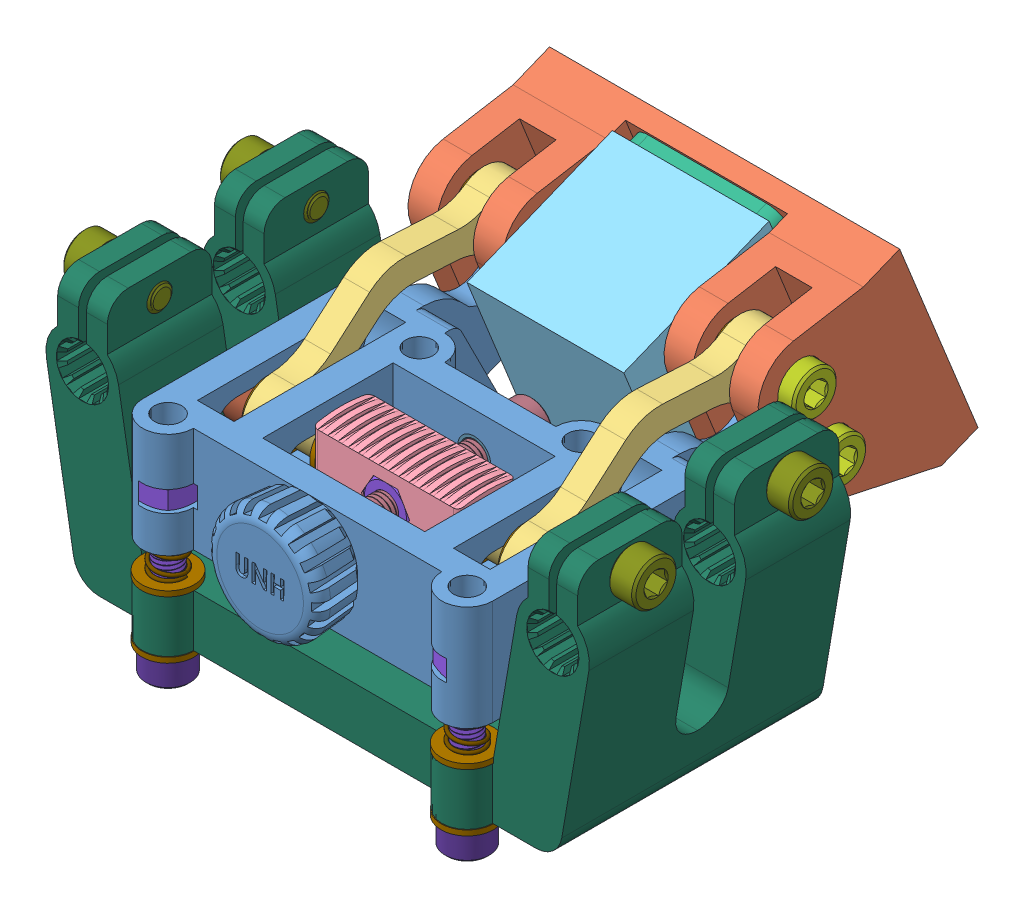
SolidWorks assembly Camera_Angle_Assembly_M5, configuration Default. Lengths in mm.
Overall size (109.96 65.35 103.86).
86 component instances, 19 part files, 86 mates.
Components (placement in the parent):
- Body_Bracket_M5-1: Body_Bracket_M5 [Default] at (-16.3834 -2.0346 -10.9973) size (67 20.14 76.95)
- Camera_Swing_Bracket_M5-1: Camera_Swing_Bracket_M5 [Default] at (-16.3834 -14.0182 -34.7174) x (1 0 0) z (0 -0.374784 0.927112) size (67 43.1 30.6)
- 42-72mm_Linkage_bent_angle_M5-1: 42-72mm_Linkage_bent_angle_M5 [Default] at (-9.8834 11.872 -5.3755) x (1 0 0) z (0 -0.325531 0.945531) size (5 16.61 54.86)
- 42-72mm_Linkage_bent_angle_M5-2: 42-72mm_Linkage_bent_angle_M5 [Default] at (-58.8834 11.872 -5.3755) x (1 0 0) z (0 -0.325531 0.945531) size (5 16.61 54.86)
- Sled_Block_M5-1: Sled_Block_M5 [Default] at (-31.8834 -2.0346 29.5176) size (28 13.83 11)
- Camera_Appr-1: Camera_Appr [Default] at (-17.3834 11.8179 9.4336) x (-1 0 0) z (0 -0.374784 0.927112) size (30 50 30)
- Adapter_Appr-1: Adapter_Appr [Default] at (-46.3834 -14.0231 -33.3711) x (0 0.927112 0.374784) z (-1 0 0) size (39 2.5 29)
- Pivot_Joints-1: Pivot_Joints [Default] at (-19.4217 -14.2043 8.9956) x (0 0.138984 0.990295) z (-1 0 0) size (10 10 21.93)
  - 16mm_M5x0-8-1: 16mm_M5x0-8 [91292A126] at (-10.6074 27.8206 -3.0383) size (8.5 8.5 21.93)
  - 8mm_M5x0-8_Nut-1: 8mm_M5x0-8_Nut [91828A241] at (-10.6074 27.8206 -5.0383) size (8 9.24 4.46)
  - 5-3_IDx10mm_OD_Washer-1: 5-3_IDx10mm_OD_Washer [93475A240] at (-10.6074 27.8206 -9.5383) size (10 10 1)
  - 5-3_IDx10mm_OD_Washer-2: 5-3_IDx10mm_OD_Washer [93475A240] at (-10.6074 27.8206 -15.5383) size (10 10 1)
  - 5mm_Bushing-1: 5mm_Bushing [Default] at (-10.6074 27.8206 -14.5383) size (6.35 6.35 5)
- Pivot_Joints-2: Pivot_Joints [Default] at (-19.4217 -28.111 3.3738) x (0 0.138984 0.990295) z (-1 0 0) size (10 10 21.93)
  - 16mm_M5x0-8-1: 16mm_M5x0-8 [91292A126] at (-10.6074 27.8206 -3.0383) size (8.5 8.5 21.93)
  - 8mm_M5x0-8_Nut-1: 8mm_M5x0-8_Nut [91828A241] at (-10.6074 27.8206 -5.0383) size (8 9.24 4.46)
  - 5-3_IDx10mm_OD_Washer-1: 5-3_IDx10mm_OD_Washer [93475A240] at (-10.6074 27.8206 -9.5383) size (10 10 1)
  - 5-3_IDx10mm_OD_Washer-2: 5-3_IDx10mm_OD_Washer [93475A240] at (-10.6074 27.8206 -15.5383) size (10 10 1)
  - 5mm_Bushing-1: 5mm_Bushing [Default] at (-10.6074 27.8206 -14.5383) size (6.35 6.35 5)
- Pivot_Joints-3: Pivot_Joints [Default] at (-44.3451 -17.1529 -12.0134) x (0 -0.138984 -0.990295) z (1 0 0) size (10 10 21.93)
  - 16mm_M5x0-8-1: 16mm_M5x0-8 [91292A126] at (-10.6074 27.8206 -3.0383) size (8.5 8.5 21.93)
  - 8mm_M5x0-8_Nut-1: 8mm_M5x0-8_Nut [91828A241] at (-10.6074 27.8206 -5.0383) size (8 9.24 4.46)
  - 5-3_IDx10mm_OD_Washer-1: 5-3_IDx10mm_OD_Washer [93475A240] at (-10.6074 27.8206 -9.5383) size (10 10 1)
  - 5-3_IDx10mm_OD_Washer-2: 5-3_IDx10mm_OD_Washer [93475A240] at (-10.6074 27.8206 -15.5383) size (10 10 1)
  - 5mm_Bushing-1: 5mm_Bushing [Default] at (-10.6074 27.8206 -14.5383) size (6.35 6.35 5)
- Pivot_Joints-4: Pivot_Joints [Default] at (-44.3451 -22.2956 10.8201) x (0 -0.927112 -0.374784) z (1 0 0) size (10 10 21.93)
  - 16mm_M5x0-8-1: 16mm_M5x0-8 [91292A126] at (-10.6074 27.8206 -3.0383) size (8.5 8.5 21.93)
  - 8mm_M5x0-8_Nut-1: 8mm_M5x0-8_Nut [91828A241] at (-10.6074 27.8206 -5.0383) size (8 9.24 4.46)
  - 5-3_IDx10mm_OD_Washer-1: 5-3_IDx10mm_OD_Washer [93475A240] at (-10.6074 27.8206 -9.5383) size (10 10 1)
  - 5-3_IDx10mm_OD_Washer-2: 5-3_IDx10mm_OD_Washer [93475A240] at (-10.6074 27.8206 -15.5383) size (10 10 1)
  - 5mm_Bushing-1: 5mm_Bushing [Default] at (-10.6074 27.8206 -14.5383) size (6.35 6.35 5)
- 8mm_M5x0-8_Nut-1: 8mm_M5x0-8_Nut [91828A241] at (-31.8834 -2.0346 38.5176) x (0.866025 -0.5 0) z (0 0 1) size (8 9.24 4.46)
- 8mm_M5x0-8_Nut-2: 8mm_M5x0-8_Nut [91828A241] at (-31.8834 -2.0346 31.5176) x (0.866025 0.5 0) z (0 0 1) size (8 9.24 4.46)
- 8mm_M5x0-8_Nut-3: 8mm_M5x0-8_Nut [91828A241] at (-43.8834 -2.0346 35.0176) x (0 -0.866025 -0.5) z (1 0 0) size (8 9.24 4.46)
- 8mm_M5x0-8_Nut-4: 8mm_M5x0-8_Nut [91828A241] at (-19.8834 -2.0346 35.0176) x (0 -0.866025 0.5) z (-1 0 0) size (8 9.24 4.46)
- 5-3_IDx10mm_OD_Washer-1: 5-3_IDx10mm_OD_Washer [93475A240] at (-31.8834 -2.0346 52.5027) x (-0.658072 -0.752955 0) z (0 0 1) size (10 10 1)
- 5-3_IDx10mm_OD_Washer-2: 5-3_IDx10mm_OD_Washer [93475A240] at (-31.8834 -2.0346 18.5527) size (10 10 1)
- Slider_Bolt_Assembly_M5-1: Slider_Bolt_Assembly_M5 [Default] at (-13.1473 -15.2033 38.4623) x (0 -0.5 0.866025) z (-1 0 0) size (13.73 13.73 25.93)
  - 20mm_M5x0-8-1: 20mm_M5x0-8 [91292A128] at (-9.5676 9.6821 10.7361) size (8.5 8.5 25.93)
  - 5-3_IDx10mm_OD_Washer-1: 5-3_IDx10mm_OD_Washer [93475A240] at (-9.5676 9.6821 -9.2639) size (10 10 1)
  - 5mm_Bushing-3: 5mm_Bushing [Default] at (-9.5676 9.6821 -8.2639) size (6.35 6.35 5)
  - 5-3_IDx10mm_OD_Washer-2: 5-3_IDx10mm_OD_Washer [93475A240] at (-9.5676 9.6821 -3.2639) x (0.855536 0.517743 0) z (0 0 1) size (10 10 1)
  - 6mm_Bushing-2: 6mm_Bushing [Default] at (-9.5676 9.6821 -2.2639) x (-0.990313 -0.138856 0) z (0 0 1) size (6.35 6.35 6)
  - 5-3_IDx10mm_OD_Washer-3: 5-3_IDx10mm_OD_Washer [93475A240] at (-9.5676 9.6821 3.7361) x (0.855536 0.517743 0) z (0 0 1) size (10 10 1)
- Slider_Bolt_Assembly_M5-2: Slider_Bolt_Assembly_M5 [Default] at (-50.6195 -11.6022 44.6996) x (0 -1 0) z (1 0 0) size (13.73 13.73 25.93)
  - 20mm_M5x0-8-1: 20mm_M5x0-8 [91292A128] at (-9.5676 9.6821 10.7361) size (8.5 8.5 25.93)
  - 5-3_IDx10mm_OD_Washer-1: 5-3_IDx10mm_OD_Washer [93475A240] at (-9.5676 9.6821 -9.2639) size (10 10 1)
  - 5mm_Bushing-3: 5mm_Bushing [Default] at (-9.5676 9.6821 -8.2639) size (6.35 6.35 5)
  - 5-3_IDx10mm_OD_Washer-2: 5-3_IDx10mm_OD_Washer [93475A240] at (-9.5676 9.6821 -3.2639) x (0.855536 0.517743 0) z (0 0 1) size (10 10 1)
  - 6mm_Bushing-2: 6mm_Bushing [Default] at (-9.5676 9.6821 -2.2639) x (-0.990313 -0.138856 0) z (0 0 1) size (6.35 6.35 6)
  - 5-3_IDx10mm_OD_Washer-3: 5-3_IDx10mm_OD_Washer [93475A240] at (-9.5676 9.6821 3.7361) x (0.855536 0.517743 0) z (0 0 1) size (10 10 1)
- 45mm_M5x0-8_Bolt-1: 45mm_M5x0-8_Bolt [91290A197] at (-31.8834 -2.0346 62.5527) x (-0.070148 -0.997537 0) z (0 0 1) size (8.5 8.5 50.62)
- 4mm_Bushing-1: 4mm_Bushing [Default] at (-31.8834 -2.0346 19.5527) x (0.999697 0.024604 0) z (0 0 1) size (6.35 6.35 4)
- 4mm_Bushing-2: 4mm_Bushing [Default] at (-31.8834 -2.0346 48.5027) x (0.999452 0.033088 0) z (0 0 1) size (6.35 6.35 4)
- 5-3_IDx10mm_OD_Washer-3: 5-3_IDx10mm_OD_Washer [93475A240] at (-31.8834 -2.0346 53.5027) x (-0.658072 -0.752955 0) z (0 0 1) size (10 10 1)
- 5-3_IDx10mm_OD_Washer-4: 5-3_IDx10mm_OD_Washer [93475A240] at (-31.8834 -2.0346 17.5527) x (-0.656863 -0.75401 0) z (0 0 1) size (10 10 1)
- Mounting_Plate_M5-1: Mounting_Plate_M5 [Default] at (-31.8834 -31.3046 30.9402) x (-1 0 0) z (0 0 -1) size (104 49.82 55.08)
- 10mm_M5x0-8_Bolt-1: 10mm_M5x0-8_Bolt [91292A124] at (7.8666 14.0165 43.5027) x (0 -0.230781 0.973006) z (-1 0 0) size (8.5 8.5 15.93)
- 10mm_M5x0-8_Bolt-2: 10mm_M5x0-8_Bolt [91292A124] at (7.8666 14.0165 13.5027) x (0 -0.230781 0.973006) z (-1 0 0) size (8.5 8.5 15.93)
- 10mm_M5x0-8_Bolt-3: 10mm_M5x0-8_Bolt [91292A124] at (-71.6334 14.0165 13.5027) x (0 -0.230781 -0.973006) z (1 0 0) size (8.5 8.5 15.93)
- 10mm_M5x0-8_Bolt-4: 10mm_M5x0-8_Bolt [91292A124] at (-71.6334 14.0165 43.5027) x (0 -0.230781 -0.973006) z (1 0 0) size (8.5 8.5 15.93)
- Spring_Tilt_Bolt-1: Spring_Tilt_Bolt [Default] at (-40.1833 -35.3156 43.4609) x (0.983923 0 -0.178593) z (0 1 0) size (11.84 12.15 35.93)
  - 30mm_M5x0-8_Bolt-1: 30mm_M5x0-8_Bolt [91292A192] at (-21.7917 -6.2505 33.0109) size (8.5 8.5 35.93)
  - 5-3_IDx10mm_OD_Washer-1: 5-3_IDx10mm_OD_Washer [93475A240] at (-21.7917 -6.2505 3.0109) size (10 10 1)
  - Spring-1: Spring [9657K272] at (-21.7731 -6.2413 27.7109) size (6.54 6.63 13.03)
  - 5-3_IDx10mm_OD_Washer-2: 5-3_IDx10mm_OD_Washer [93475A240] at (-21.7917 -6.2505 14.0109) x (0.999587 -0.028726 0) z (0 0 1) size (10 10 1)
  - 8mm_M5x0-8_Nut-1: 8mm_M5x0-8_Nut [91828A241] at (-21.7917 -6.2505 29.7109) x (0.822023 0.569454 0) z (0 0 1) size (8 9.24 4.46)
- Spring_Tilt_Bolt-2: Spring_Tilt_Bolt [Default] at (-13.3002 -35.3156 33.1776) x (-0.178593 0 -0.983923) z (0 1 0) size (11.84 12.15 35.93)
  - 30mm_M5x0-8_Bolt-1: 30mm_M5x0-8_Bolt [91292A192] at (-21.7917 -6.2505 33.0109) size (8.5 8.5 35.93)
  - 5-3_IDx10mm_OD_Washer-1: 5-3_IDx10mm_OD_Washer [93475A240] at (-21.7917 -6.2505 3.0109) size (10 10 1)
  - Spring-1: Spring [9657K272] at (-21.7731 -6.2413 27.7109) size (6.54 6.63 13.03)
  - 5-3_IDx10mm_OD_Washer-2: 5-3_IDx10mm_OD_Washer [93475A240] at (-21.7917 -6.2505 14.0109) x (0.999587 -0.028726 0) z (0 0 1) size (10 10 1)
  - 8mm_M5x0-8_Nut-1: 8mm_M5x0-8_Nut [91828A241] at (-21.7917 -6.2505 29.7109) x (0.822023 0.569454 0) z (0 0 1) size (8 9.24 4.46)
- Spring_Tilt_Bolt-3: Spring_Tilt_Bolt [Default] at (-25.9107 -35.3156 25.8241) x (0.822023 0 0.569454) z (0 1 0) size (11.84 12.15 35.93)
  - 30mm_M5x0-8_Bolt-1: 30mm_M5x0-8_Bolt [91292A192] at (-21.7917 -6.2505 33.0109) size (8.5 8.5 35.93)
  - 5-3_IDx10mm_OD_Washer-1: 5-3_IDx10mm_OD_Washer [93475A240] at (-21.7917 -6.2505 3.0109) size (10 10 1)
  - Spring-1: Spring [9657K272] at (-21.7731 -6.2413 27.7109) size (6.54 6.63 13.03)
  - 5-3_IDx10mm_OD_Washer-2: 5-3_IDx10mm_OD_Washer [93475A240] at (-21.7917 -6.2505 14.0109) x (0.999587 -0.028726 0) z (0 0 1) size (10 10 1)
  - 8mm_M5x0-8_Nut-1: 8mm_M5x0-8_Nut [91828A241] at (-21.7917 -6.2505 29.7109) x (0.822023 0.569454 0) z (0 0 1) size (8 9.24 4.46)
- Spring_Tilt_Bolt-4: Spring_Tilt_Bolt [Default] at (-20.8225 -35.3156 -3.6789) x (0.082151 0 -0.99662) z (0 1 0) size (11.84 12.15 35.93)
  - 30mm_M5x0-8_Bolt-1: 30mm_M5x0-8_Bolt [91292A192] at (-21.7917 -6.2505 33.0109) size (8.5 8.5 35.93)
  - 5-3_IDx10mm_OD_Washer-1: 5-3_IDx10mm_OD_Washer [93475A240] at (-21.7917 -6.2505 3.0109) size (10 10 1)
  - Spring-1: Spring [9657K272] at (-21.7731 -6.2413 27.7109) size (6.54 6.63 13.03)
  - 5-3_IDx10mm_OD_Washer-2: 5-3_IDx10mm_OD_Washer [93475A240] at (-21.7917 -6.2505 14.0109) x (0.999587 -0.028726 0) z (0 0 1) size (10 10 1)
  - 8mm_M5x0-8_Nut-1: 8mm_M5x0-8_Nut [91828A241] at (-21.7917 -6.2505 29.7109) x (0.822023 0.569454 0) z (0 0 1) size (8 9.24 4.46)
- Knob-1: Knob [Default] at (-31.8834 -2.0346 54.5027) x (0.999929 -0.011934 0) z (0 0 1) size (21.77 21.77 10)
Mates (geometry in assembly coordinates):
- Distance2: distance = 1 mm anti-aligned: plane of Camera_Swing_Bracket_M5-1 through (-10.8834 -14.0182 -34.7174) normal (1 0 0); plane of Body_Bracket_M5-1 through (-9.8834 -2.0346 -10.9973) normal (-1 0 0)
- Distance3: distance = 1 mm anti-aligned: plane of 42-72mm_Linkage_bent_angle_M5-1 through (-4.8834 14.025 35.5957) normal (1 0 0); plane of Camera_Swing_Bracket_M5-1 through (-3.8834 -14.0182 -34.7174) normal (-1 0 0)
- Slot1: slot aligned: cylinder of 42-72mm_Linkage_bent_angle_M5-1 through (-4.8834 -2.0346 35.0176) axis (-1 0 0) radius 3.175; plane of Body_Bracket_M5-1 through (1.6166 -5.2096 41.0027) normal (0 1 0); cylinder of Body_Bracket_M5-1 through (1.6166 -2.0346 29.0027) axis (-1 0 0) radius 3.175
- Concentric3: concentric anti-aligned: circle of Camera_Swing_Bracket_M5-1; circle of 42-72mm_Linkage_bent_angle_M5-2
- Concentric4: concentric aligned: circle of 42-72mm_Linkage_bent_angle_M5-1; circle of 42-72mm_Linkage_bent_angle_M5-2
- Distance4: distance = 1 mm anti-aligned: plane of 42-72mm_Linkage_bent_angle_M5-2 through (-58.8834 14.025 35.5957) normal (-1 0 0); plane of Camera_Swing_Bracket_M5-1 through (-59.8834 -14.0182 -34.7174) normal (1 0 0)
- Concentric6: concentric anti-aligned: circle of Body_Bracket_M5-1; circle of Sled_Block_M5-1
- Concentric7: concentric anti-aligned: circle of Camera_Swing_Bracket_M5-1; circle of Adapter_Appr-1
- Parallel1: parallel anti-aligned: plane of Camera_Swing_Bracket_M5-1 through (1.6166 -2.0346 -10.9973) normal (1 0 0); plane of Adapter_Appr-1 through (-46.3834 -10.1194 -34.4896) normal (-1 0 0)
- Coincident1: coincident anti-aligned: plane of Camera_Swing_Bracket_M5-1 through (-31.8834 -13.5497 -35.8763) normal (0 -0.374784 0.927112); plane of Adapter_Appr-1 through (-43.1834 -10.1194 -34.4896) normal (0 0.374784 -0.927112)
- Coincident2: coincident anti-aligned: plane of Camera_Appr-1 through (-17.3834 -14.0231 -33.3711) normal (0 0.374784 -0.927112); plane of Adapter_Appr-1 through (-43.1834 -11.0563 -32.1718) normal (0 -0.374784 0.927112)
- Coincident3: coincident aligned: plane of Camera_Appr-1 through (-17.3834 -25.2666 -5.5578) normal (1 0 0); plane of Adapter_Appr-1 through (-17.3834 -10.1194 -34.4896) normal (1 0 0)
- Coincident4: coincident aligned: plane of Camera_Appr-1 through (-17.3834 -25.2666 -5.5578) normal (0 -0.927112 -0.374784); plane of Adapter_Appr-1 through (-43.1834 -13.0861 -35.6889) normal (0 -0.927112 -0.374784)
- LimitAngle3: limit planar angle = 1.95496 rad anti-aligned: plane of Camera_Swing_Bracket_M5-1 through (1.6166 -12.1443 -39.353) normal (0 0.374784 -0.927112); plane of Body_Bracket_M5-1 through (1.6166 5.5354 13.4839) normal (0 1 0)
- Concentric8: concentric aligned: circle of Camera_Swing_Bracket_M5-1; circle of 42-72mm_Linkage_bent_angle_M5-1
- Concentric9: concentric aligned: circle of Body_Bracket_M5-1; circle of Camera_Swing_Bracket_M5-1
- Concentric10: concentric anti-aligned: circle of Camera_Swing_Bracket_M5-1; circle of Pivot_Joints-1/5-3_IDx10mm_OD_Washer-2
- Coincident5: coincident anti-aligned: plane of Camera_Swing_Bracket_M5-1 through (-0.3834 11.872 -5.3755) normal (1 0 0); plane of Pivot_Joints-1/16mm_M5x0-8-1 through (-0.3834 11.872 -5.3755) normal (-1 0 0)
- Coincident6: coincident anti-aligned: plane of Camera_Swing_Bracket_M5-1 through (-12.3834 13.6031 -9.6577) normal (0 -0.788128 0.615511); plane of Pivot_Joints-1/8mm_M5x0-8_Nut-1 through (-16.3834 16.446 -6.0175) normal (0 0.788128 -0.615511)
- Concentric11: concentric aligned: circle of Camera_Swing_Bracket_M5-1; circle of Pivot_Joints-2/16mm_M5x0-8-1
- Coincident7: coincident anti-aligned: circle of Camera_Swing_Bracket_M5-1; plane of Pivot_Joints-2/16mm_M5x0-8-1 through (-0.3834 -2.0346 -10.9973) normal (-1 0 0)
- Parallel2: parallel anti-aligned: plane of Camera_Swing_Bracket_M5-1 through (-12.3834 -4.8776 -14.6375) normal (0 0.138984 0.990295); plane of Pivot_Joints-2/8mm_M5x0-8_Nut-1 through (-16.3834 -0.3036 -15.2794) normal (0 -0.138984 -0.990295)
- Concentric12: concentric aligned: circle of Camera_Swing_Bracket_M5-1; circle of Pivot_Joints-3/5-3_IDx10mm_OD_Washer-2
- Coincident8: coincident anti-aligned: plane of Camera_Swing_Bracket_M5-1 through (-63.3834 11.872 -5.3755) normal (-1 0 0); plane of Pivot_Joints-3/16mm_M5x0-8-1 through (-63.3834 11.872 -5.3755) normal (1 0 0)
- Parallel3: parallel anti-aligned: plane of Camera_Swing_Bracket_M5-1 through (-51.3834 13.6031 -9.6577) normal (0 -0.788128 0.615511); plane of Pivot_Joints-3/8mm_M5x0-8_Nut-1 through (-47.3834 13.6031 -9.6577) normal (0 0.788128 -0.615511)
- Concentric13: concentric aligned: circle of Camera_Swing_Bracket_M5-1; circle of Pivot_Joints-4/5-3_IDx10mm_OD_Washer-2
- Coincident9: coincident anti-aligned: plane of Camera_Swing_Bracket_M5-1 through (-63.3834 -2.0346 -10.9973) normal (-1 0 0); plane of Pivot_Joints-4/16mm_M5x0-8-1 through (-63.3834 -2.0346 -10.9973) normal (1 0 0)
- Parallel4: parallel anti-aligned: plane of Camera_Swing_Bracket_M5-1 through (-51.3834 -0.3036 -15.2794) normal (0 -0.788128 0.615511); plane of Pivot_Joints-4/8mm_M5x0-8_Nut-1 through (-47.3834 -0.3036 -15.2794) normal (0 0.788128 -0.615511)
- Concentric14: concentric anti-aligned: circle of 42-72mm_Linkage_bent_angle_M5-1; circle of Sled_Block_M5-1
- Parallel5: parallel anti-aligned: plane of Sled_Block_M5-1 through (-27.2646 -2.0346 36.5176) normal (-0.866025 -0.5 0); plane of 8mm_M5x0-8_Nut-1 through (-27.2646 -2.0346 40.5176) normal (0.866025 0.5 0)
- Coincident10: coincident anti-aligned: plane of Sled_Block_M5-1 through (-27.2646 -2.0346 36.5176) normal (-0.866025 -0.5 0); plane of 8mm_M5x0-8_Nut-1 through (-27.2646 -2.0346 40.5176) normal (0.866025 0.5 0)
- Concentric15: concentric anti-aligned: circle of Sled_Block_M5-1; circle of 8mm_M5x0-8_Nut-1
- Coincident11: coincident anti-aligned: plane of Sled_Block_M5-1 through (-31.8834 -2.0346 36.5176) normal (0 0 1); plane of 8mm_M5x0-8_Nut-1 through (-34.1928 1.9654 36.5176) normal (0 0 -1)
- Parallel6: parallel anti-aligned: plane of Sled_Block_M5-1 through (-34.1928 1.9654 33.5176) normal (0.866025 -0.5 0); plane of 8mm_M5x0-8_Nut-2 through (-34.1928 1.9654 33.5176) normal (-0.866025 0.5 0)
- Concentric16: concentric aligned: circle of Sled_Block_M5-1; circle of 8mm_M5x0-8_Nut-2
- Coincident12: coincident aligned: plane of Sled_Block_M5-1 through (-31.8834 -2.0346 29.5176) normal (0 0 -1); plane of 8mm_M5x0-8_Nut-2 through (-36.5022 -2.0346 29.5176) normal (0 0 -1)
- Coincident13: coincident anti-aligned: plane of Sled_Block_M5-1 through (-41.8834 -2.0346 29.5176) normal (-1 0 0); plane of 8mm_M5x0-8_Nut-3 through (-41.8834 2.5842 35.0176) normal (1 0 0)
- Parallel7: parallel aligned: plane of Sled_Block_M5-1 through (-41.8834 -6.6534 35.0176) normal (0 0.866025 -0.5); plane of 8mm_M5x0-8_Nut-3 through (-41.8834 0.2748 31.0176) normal (0 0.866025 -0.5)
- Concentric17: concentric anti-aligned: circle of Sled_Block_M5-1; circle of 8mm_M5x0-8_Nut-3
- Coincident14: coincident anti-aligned: plane of Sled_Block_M5-1 through (-21.8834 -2.0346 29.5176) normal (1 0 0); plane of 8mm_M5x0-8_Nut-4 through (-21.8834 2.5842 35.0176) normal (-1 0 0)
- Parallel8: parallel aligned: plane of Sled_Block_M5-1 through (-21.8834 0.2748 31.0176) normal (0 0 1); plane of 8mm_M5x0-8_Nut-4 through (-21.8834 -4.344 39.0176) normal (0 0 1)
- Concentric18: concentric anti-aligned: circle of Sled_Block_M5-1; circle of 8mm_M5x0-8_Nut-4
- Coincident15: coincident anti-aligned: plane of Body_Bracket_M5-1 through (-31.8834 -2.0346 52.5027) normal (0 0 1); plane of 5-3_IDx10mm_OD_Washer-1 through (-31.8834 -2.0346 52.5027) normal (0 0 -1)
- Concentric19: concentric aligned: circle of Body_Bracket_M5-1; circle of 5-3_IDx10mm_OD_Washer-1
- Coincident16: coincident anti-aligned: plane of Body_Bracket_M5-1 through (-31.8834 -2.0346 19.5527) normal (0 0 -1); plane of 5-3_IDx10mm_OD_Washer-2 through (-31.8834 -2.0346 19.5527) normal (0 0 1)
- Concentric20: concentric anti-aligned: circle of Body_Bracket_M5-1; circle of 5-3_IDx10mm_OD_Washer-2
- Concentric21: concentric anti-aligned: circle of 42-72mm_Linkage_bent_angle_M5-1; circle of Slider_Bolt_Assembly_M5-1/20mm_M5x0-8-1
- Coincident17: coincident anti-aligned: plane of 42-72mm_Linkage_bent_angle_M5-1 through (-4.8834 14.025 35.5957) normal (1 0 0); plane of Slider_Bolt_Assembly_M5-1/5-3_IDx10mm_OD_Washer-1 through (-4.8834 -2.0346 35.0176) normal (-1 0 0)
- Concentric22: concentric aligned: circle of 42-72mm_Linkage_bent_angle_M5-2; circle of Slider_Bolt_Assembly_M5-2/20mm_M5x0-8-1
- Coincident18: coincident anti-aligned: plane of 42-72mm_Linkage_bent_angle_M5-2 through (-58.8834 14.025 35.5957) normal (-1 0 0); plane of Slider_Bolt_Assembly_M5-2/5-3_IDx10mm_OD_Washer-1 through (-58.8834 -2.0346 35.0176) normal (1 0 0)
- Parallel9: parallel aligned: plane of Body_Bracket_M5-1 through (-37.364 -6.4096 29.0027) normal (0 1 0); plane of Slider_Bolt_Assembly_M5-2/20mm_M5x0-8-1 through (-61.8834 -4.0346 33.8629) normal (0 1 0)
- Parallel10: parallel aligned: plane of Body_Bracket_M5-1 through (-26.4028 -6.4096 29.0027) normal (0 1 0); plane of Slider_Bolt_Assembly_M5-1/20mm_M5x0-8-1 through (-1.8834 -4.0346 36.1723) normal (0 1 0)
- Concentric23: concentric aligned: circle of 5-3_IDx10mm_OD_Washer-2; circle of 45mm_M5x0-8_Bolt-1
- Concentric24: concentric aligned: circle of 5-3_IDx10mm_OD_Washer-2; circle of 4mm_Bushing-1
- Coincident20: coincident anti-aligned: plane of 5-3_IDx10mm_OD_Washer-2 through (-31.8834 -2.0346 19.5527) normal (0 0 1); plane of 4mm_Bushing-1 through (-31.8834 -2.0346 19.5527) normal (0 0 -1)
- Concentric25: concentric aligned: circle of 5-3_IDx10mm_OD_Washer-1; circle of 4mm_Bushing-2
- Coincident21: coincident anti-aligned: plane of 5-3_IDx10mm_OD_Washer-1 through (-31.8834 -2.0346 52.5027) normal (0 0 -1); plane of 4mm_Bushing-2 through (-31.8834 -2.0346 52.5027) normal (0 0 1)
- Concentric26: concentric aligned: circle of Body_Bracket_M5-1; circle of 5-3_IDx10mm_OD_Washer-3
- Coincident22: coincident anti-aligned: plane of 5-3_IDx10mm_OD_Washer-1 through (-31.8834 -2.0346 53.5027) normal (0 0 1); plane of 5-3_IDx10mm_OD_Washer-3 through (-31.8834 -2.0346 53.5027) normal (0 0 -1)
- Concentric29: concentric anti-aligned: circle of 45mm_M5x0-8_Bolt-1; circle of 5-3_IDx10mm_OD_Washer-4
- Coincident24: coincident anti-aligned: plane of Body_Bracket_M5-1 through (-31.8834 21.8219 18.5527) normal (0 0 -1); plane of 5-3_IDx10mm_OD_Washer-4 through (-31.8834 -2.0346 18.5527) normal (0 0 1)
- Coincident25: coincident anti-aligned: plane of 45mm_M5x0-8_Bolt-1 through (-31.8834 -2.0346 17.5527) normal (0 0 1); plane of 5-3_IDx10mm_OD_Washer-4 through (-31.8834 -2.0346 17.5527) normal (0 0 -1)
- Concentric33: concentric aligned: circle of Body_Bracket_M5-1; circle of Mounting_Plate_M5-1
- Concentric34: concentric aligned: circle of Body_Bracket_M5-1; circle of Mounting_Plate_M5-1
- Concentric35: concentric anti-aligned: circle of Mounting_Plate_M5-1; circle of 10mm_M5x0-8_Bolt-1
- Coincident29: coincident anti-aligned: plane of Mounting_Plate_M5-1 through (17.8666 9.5165 -49.6423) normal (1 0 0); plane of 10mm_M5x0-8_Bolt-1 through (17.8666 14.0165 43.5027) normal (-1 0 0)
- Concentric36: concentric aligned: circle of Mounting_Plate_M5-1; circle of 10mm_M5x0-8_Bolt-2
- Coincident30: coincident anti-aligned: plane of Mounting_Plate_M5-1 through (17.8666 9.5165 -49.6423) normal (1 0 0); plane of 10mm_M5x0-8_Bolt-2 through (17.8666 14.0165 13.5027) normal (-1 0 0)
- Concentric37: concentric aligned: circle of Mounting_Plate_M5-1; circle of 10mm_M5x0-8_Bolt-3
- Coincident31: coincident anti-aligned: plane of Mounting_Plate_M5-1 through (-81.6334 17.5165 -49.6423) normal (-1 0 0); plane of 10mm_M5x0-8_Bolt-3 through (-81.6334 14.0165 13.5027) normal (1 0 0)
- Concentric38: concentric aligned: circle of Mounting_Plate_M5-1; circle of 10mm_M5x0-8_Bolt-4
- Coincident32: coincident anti-aligned: plane of Mounting_Plate_M5-1 through (-81.6334 17.5165 -49.6423) normal (-1 0 0); plane of 10mm_M5x0-8_Bolt-4 through (-81.6334 14.0165 43.5027) normal (1 0 0)
- Concentric39: concentric anti-aligned: circle of Mounting_Plate_M5-1; circle of Spring_Tilt_Bolt-1/5-3_IDx10mm_OD_Washer-1
- Coincident34: coincident anti-aligned: plane of Mounting_Plate_M5-1 through (-60.5084 -31.3046 53.5027) normal (0 -1 0); plane of Spring_Tilt_Bolt-1/5-3_IDx10mm_OD_Washer-1 through (-60.5084 -31.3046 53.5027) normal (0 1 0)
- Parallel15: parallel anti-aligned: plane of Body_Bracket_M5-1 through (-59.313 -7.6046 49.0413) normal (-0.707107 0 0.707107); plane of Spring_Tilt_Bolt-1/8mm_M5x0-8_Nut-1 through (-56.047 -3.6046 52.3073) normal (0.707107 0 -0.707107)
- Coincident35: coincident anti-aligned: plane of Body_Bracket_M5-1 through (-16.3834 -3.6046 -10.9973) normal (0 -1 0); plane of Spring_Tilt_Bolt-1/8mm_M5x0-8_Nut-1 through (-64.9698 -3.6046 54.6981) normal (0 1 0)
- Concentric40: concentric aligned: circle of Mounting_Plate_M5-1; circle of Spring_Tilt_Bolt-2/5-3_IDx10mm_OD_Washer-1
- Coincident36: coincident anti-aligned: plane of Mounting_Plate_M5-1 through (-60.5084 -31.3046 53.5027) normal (0 -1 0); plane of Spring_Tilt_Bolt-2/5-3_IDx10mm_OD_Washer-1 through (-3.2584 -31.3046 53.5027) normal (0 1 0)
- Parallel16: parallel aligned: plane of Body_Bracket_M5-1 through (-4.4538 -7.6046 49.0413) normal (0.707107 0 0.707107); plane of Spring_Tilt_Bolt-2/8mm_M5x0-8_Nut-1 through (-2.063 -3.6046 57.9641) normal (0.707107 0 0.707107)
- Concentric41: concentric aligned: circle of Mounting_Plate_M5-1; circle of Spring_Tilt_Bolt-3/5-3_IDx10mm_OD_Washer-1
- Coincident37: coincident anti-aligned: plane of Mounting_Plate_M5-1 through (-60.5084 -31.3046 53.5027) normal (0 -1 0); plane of Spring_Tilt_Bolt-3/5-3_IDx10mm_OD_Washer-1 through (-47.3834 -31.3046 18.5527) normal (0 1 0)
- Parallel17: parallel anti-aligned: plane of Body_Bracket_M5-1 through (-38.5382 -7.6046 18.0647) normal (-0.5 0 -0.866025); plane of Spring_Tilt_Bolt-3/8mm_M5x0-8_Nut-1 through (-47.3834 -3.6046 23.1715) normal (0.5 0 0.866025)
- Concentric42: concentric aligned: circle of Mounting_Plate_M5-1; circle of Spring_Tilt_Bolt-4/5-3_IDx10mm_OD_Washer-1
- Coincident38: coincident anti-aligned: plane of Mounting_Plate_M5-1 through (-60.5084 -31.3046 53.5027) normal (0 -1 0); plane of Spring_Tilt_Bolt-4/5-3_IDx10mm_OD_Washer-1 through (-16.3834 -31.3046 18.5527) normal (0 1 0)
- Parallel18: parallel anti-aligned: plane of Body_Bracket_M5-1 through (-25.2286 -7.6046 18.0647) normal (0.5 0 -0.866025); plane of Spring_Tilt_Bolt-4/8mm_M5x0-8_Nut-1 through (-20.3834 -3.6046 20.8621) normal (-0.5 0 0.866025)
- Coincident39: coincident anti-aligned: circle of 5-3_IDx10mm_OD_Washer-3; plane of Knob-1 through (-31.8834 -2.0346 54.5027) normal (0 0 -1)
